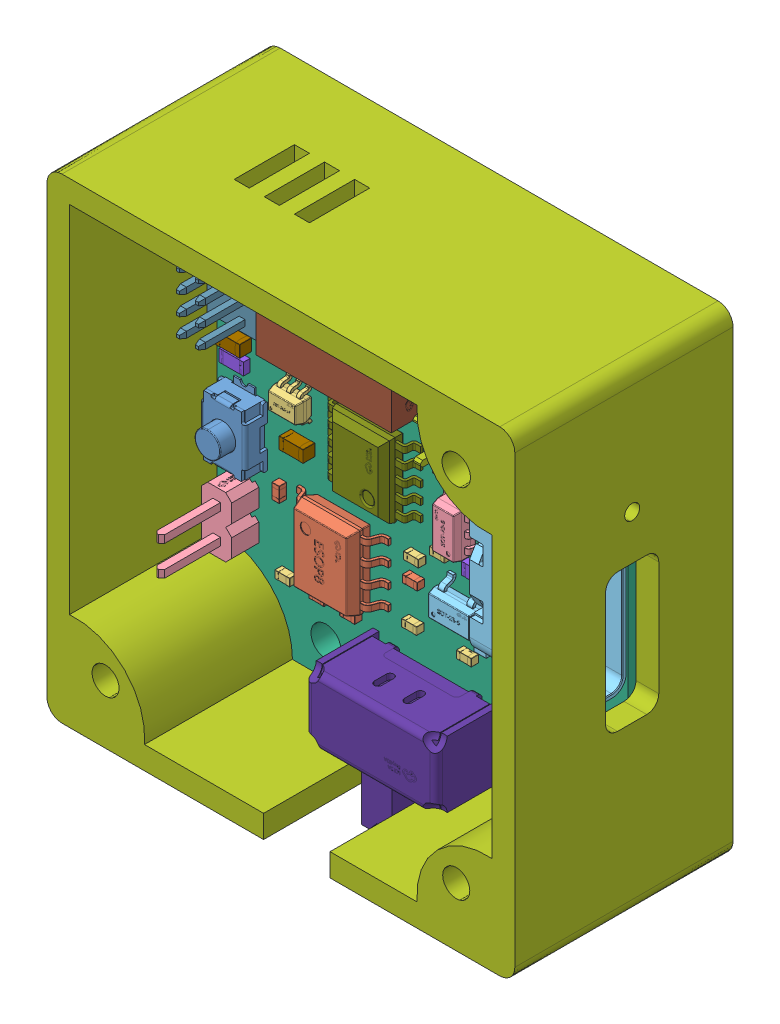
SolidWorks assembly 3D_PCB4_2025-05-12, configuration 默认. Lengths in mm.
Overall size (31.09 33.6 14.5).
127 component instances, 26 part files, 3 mates.
Components (placement in the parent):
- 3D_PCB4_2025-05-12.step-1: 3D_PCB4_2025-05-12.step [默认] at origin size (27.28 31.7 8.7)
  - D4.step-1: D4.step [默认] at (16.256 -9.9568 1.5862) x (-1 0 0) z (0 0 1) size (3.7 1.8 1.14)
    - SOD-123FL_L2.8-W1.8-LS3.7-BI.step-1: SOD-123FL_L2.8-W1.8-LS3.7-BI.step [默认] at origin size (3.7 1.8 1.14)
      - SOLID.step-1: SOLID.step [默认] at origin size (3.7 1.8 1.14)
  - R1.step-1: R1.step [默认] at (4.3814 -18.288 1.5862) x (0 1 0) z (0 0 1) size (1 0.5 0.5)
    - R0402.step-1: R0402.step [默认] at origin size (1 0.5 0.5)
      - SOLID-0.step-1: SOLID-0.step [默认] at origin size (1 0.5 0.5)
  - R2.step-1: R2.step [默认] at (13.305 -18.9963 1.5862) x (-1 0 0) z (0 0 1) size (1 0.5 0.5)
    - R0402.step-1: R0402.step [默认] at origin size (1 0.5 0.5)
      - SOLID-0.step-1: SOLID-0.step [默认] at origin size (1 0.5 0.5)
  - R3.step-1: R3.step [默认] at (20.701 -24.257 1.5862) x (0 -1 0) z (0 0 1) size (1 0.5 0.5)
    - R0402.step-1: R0402.step [默认] at origin size (1 0.5 0.5)
      - SOLID-0.step-1: SOLID-0.step [默认] at origin size (1 0.5 0.5)
  - R4.step-1: R4.step [默认] at (20.701 -26.4161 1.5862) x (0 -1 0) z (0 0 1) size (1 0.5 0.5)
    - R0402.step-1: R0402.step [默认] at origin size (1 0.5 0.5)
      - SOLID-0.step-1: SOLID-0.step [默认] at origin size (1 0.5 0.5)
  - R5.step-1: R5.step [默认] at (7.1031 -22.987 1.5862) size (1 0.5 0.5)
    - R0402.step-1: R0402.step [默认] at origin size (1 0.5 0.5)
      - SOLID-0.step-1: SOLID-0.step [默认] at origin size (1 0.5 0.5)
  - R6.step-1: R6.step [默认] at (9.144 -22.987 1.5862) size (1 0.5 0.5)
    - R0402.step-1: R0402.step [默认] at origin size (1 0.5 0.5)
      - SOLID-0.step-1: SOLID-0.step [默认] at origin size (1 0.5 0.5)
  - R7.step-1: R7.step [默认] at (15.5701 -5.9643 1.5862) x (-1 0 0) z (0 0 1) size (1 0.5 0.5)
    - R0402.step-1: R0402.step [默认] at origin size (1 0.5 0.5)
      - SOLID-0.step-1: SOLID-0.step [默认] at origin size (1 0.5 0.5)
  - R8.step-1: R8.step [默认] at (15.5701 -7.3615 1.5862) x (-1 0 0) z (0 0 1) size (1 0.5 0.5)
    - R0402.step-1: R0402.step [默认] at origin size (1 0.5 0.5)
      - SOLID-0.step-1: SOLID-0.step [默认] at origin size (1 0.5 0.5)
  - C1.step-1: C1.step [默认] at (13.3845 -17.6277 1.5862) x (-1 0 0) z (0 0 1) size (1 0.5 0.5)
    - C0402.step-1: C0402.step [默认] at origin size (1 0.5 0.5)
      - SOLID-1.step-1: SOLID-1.step [默认] at origin size (1 0.5 0.5)
  - C2.step-1: C2.step [默认] at (13.2575 -21.5647 1.5862) x (-1 0 0) z (0 0 1) size (1 0.5 0.5)
    - C0402.step-1: C0402.step [默认] at origin size (1 0.5 0.5)
      - SOLID-1.step-1: SOLID-1.step [默认] at origin size (1 0.5 0.5)
  - C3.step-1: C3.step [默认] at (21.847 -24.257 1.5862) x (0 1 0) z (0 0 1) size (1 0.5 0.5)
    - C0402.step-1: C0402.step [默认] at origin size (1 0.5 0.5)
      - SOLID-1.step-1: SOLID-1.step [默认] at origin size (1 0.5 0.5)
  - C20.step-1: C20.step [默认] at (16.891 -21.5647 1.5862) size (1 0.5 0.5)
    - C0402.step-1: C0402.step [默认] at origin size (1 0.5 0.5)
      - SOLID-1.step-1: SOLID-1.step [默认] at origin size (1 0.5 0.5)
  - C6.step-1: C6.step [默认] at (26.0351 -20.8598 1.5862) x (0 1 0) z (0 0 1) size (1 0.5 0.5)
    - C0402.step-1: C0402.step [默认] at origin size (1 0.5 0.5)
      - SOLID-1.step-1: SOLID-1.step [默认] at origin size (1 0.5 0.5)
  - C7.step-1: C7.step [默认] at (4.826 -22.987 1.5862) x (-1 0 0) z (0 0 1) size (1 0.5 0.5)
    - C0402.step-1: C0402.step [默认] at origin size (1 0.5 0.5)
      - SOLID-1.step-1: SOLID-1.step [默认] at origin size (1 0.5 0.5)
  - C21.step-1: C21.step [默认] at (15.113 -16.4846 1.5862) size (1 0.5 0.5)
    - C0402.step-1: C0402.step [默认] at origin size (1 0.5 0.5)
      - SOLID-1.step-1: SOLID-1.step [默认] at origin size (1 0.5 0.5)
  - H3.step-1: H3.step [默认] at (1.778 -20.6168 1.5862) x (0 1 0) z (0 0 1) size (4.01 2 8.7)
    - HDR-TH_2P-P2.00-V-M.step-1: HDR-TH_2P-P2.00-V-M.step [默认] at origin size (4.01 2 8.7)
      - SOLID-2.step-1: SOLID-2.step [默认] at origin size (4.01 2 8.7)
  - U11.step-1: U11.step [默认] at (16.637 -18.921 1.5862) size (2.9 3.01 1.25)
    - SOT-23-5_L3.0-W1.7-P0.95-LS2.8-BL.step-1: SOT-23-5_L3.0-W1.7-P0.95-LS2.8-BL.step [默认] at origin size (2.9 3.01 1.25)
      - COMPOUND.step-1: COMPOUND.step [默认] at origin size (2.9 3.01 1.25)
  - U9.step-1: U9.step [默认] at (24.892 -7.874 1.5862) x (-1 0 0) z (0 0 1) size (2.1 1.4 0.8)
    - F0805.step-1: F0805.step [默认] at origin size (2.1 1.4 0.8)
      - SOLID-3.step-1: SOLID-3.step [默认] at origin size (2.1 1.4 0.8)
  - H2.step-1: H2.step [默认] at (19.8587 -5.334 1.5862) size (5.09 2 7.2)
    - HDR-TH_4P-P1.27-V-M.step-1: HDR-TH_4P-P1.27-V-M.step [默认] at origin size (5.09 2 7.2)
      - SOLID-4.step-1: SOLID-4.step [默认] at origin size (5.09 2 7.2)
  - H4.step-1: H4.step [默认] at (19.8864 -7.6708 1.5862) size (5.09 2 7.2)
    - HDR-TH_4P-P1.27-V-M.step-1: HDR-TH_4P-P1.27-V-M.step [默认] at origin size (5.09 2 7.2)
      - SOLID-4.step-1: SOLID-4.step [默认] at origin size (5.09 2 7.2)
  - R12.step-1: R12.step [默认] at (17.4966 -16.4846 1.5862) x (-1 0 0) z (0 0 1) size (1.62 0.81 0.45)
    - R0402-1.step-1: R0402-1.step [默认] at origin size (1.62 0.81 0.45)
      - COMPOUND-5.step-1: COMPOUND-5.step [默认] at origin size (1.62 0.81 0.45)
  - R13.step-1: R13.step [默认] at (16.7346 -11.7094 1.5862) x (-1 0 0) z (0 0 1) size (1.62 0.81 0.45)
    - R0402-1.step-1: R0402-1.step [默认] at origin size (1.62 0.81 0.45)
      - COMPOUND-5.step-1: COMPOUND-5.step [默认] at origin size (1.62 0.81 0.45)
  - R14.step-1: R14.step [默认] at (1.397 -12.2844 1.5862) size (1.62 0.81 0.45)
    - R0402-1.step-1: R0402-1.step [默认] at origin size (1.62 0.81 0.45)
      - COMPOUND-5.step-1: COMPOUND-5.step [默认] at origin size (1.62 0.81 0.45)
  - C12.step-1: C12.step [默认] at (1.5009 -11.049 1.5862) x (-1 0 0) z (0 0 1) size (1.6 0.8 0.8)
    - C0402-1.step-1: C0402-1.step [默认] at origin size (1.6 0.8 0.8)
      - SOLID-6.step-1: SOLID-6.step [默认] at origin size (1.6 0.8 0.8)
  - C22.step-1: C22.step [默认] at (5.715 -14.986 1.5862) x (-1 0 0) z (0 0 1) size (1.6 0.8 0.8)
    - C0402-1.step-1: C0402-1.step [默认] at origin size (1.6 0.8 0.8)
      - SOLID-6.step-1: SOLID-6.step [默认] at origin size (1.6 0.8 0.8)
  - D3.step-1: D3.step [默认] at (15.4432 -1.0668 1.5862) size (2.5 1.25 0.95)
    - SOD-323_L1.7-W1.3-LS2.5-FD.step-1: SOD-323_L1.7-W1.3-LS2.5-FD.step [默认] at origin size (2.5 1.25 0.95)
      - COMPOUND-7.step-1: COMPOUND-7.step [默认] at origin size (2.5 1.25 0.95)
  - BUZZER.step-1: BUZZER.step [默认] at (8.89 -5.179 1.5862) x (0 -1 0) z (0 0 1) size (9 9.01 1.81)
    - BUZ-SMD_L9.0-W9.0-P8.00-LS9.3.step-1: BUZ-SMD_L9.0-W9.0-P8.00-LS9.3.step [默认] at origin size (9 9.01 1.81)
      - SOLID-8.step-1: SOLID-8.step [默认] at origin size (9 9.01 1.81)
  - D1.step-1: D1.step [默认] at (24.3141 -21.0153 1.5862) x (0 -1 0) z (0 0 1) size (2.65 1.3 0.95)
    - SOD-323_L1.8-W1.3-LS2.5-RD.step-1: SOD-323_L1.8-W1.3-LS2.5-RD.step [默认] at origin size (2.65 1.3 0.95)
      - SOLID-9.step-1: SOLID-9.step [默认] at origin size (2.65 1.3 0.95)
  - D2.step-1: D2.step [默认] at (22.5852 -21.0153 1.5862) x (0 -1 0) z (0 0 1) size (2.65 1.3 0.95)
    - SOD-323_L1.8-W1.3-LS2.5-RD.step-1: SOD-323_L1.8-W1.3-LS2.5-RD.step [默认] at origin size (2.65 1.3 0.95)
      - SOLID-9.step-1: SOLID-9.step [默认] at origin size (2.65 1.3 0.95)
  - LED1.step-1: LED1.step [默认] at (24.8995 -5.8674 1.5862) size (1 0.51 0.41)
    - LED_0402.step-1: LED_0402.step [默认] at origin size (1 0.51 0.41)
      - COMPOUND-10.step-1: COMPOUND-10.step [默认] at origin size (1 0.51 0.41)
  - U6.step-1: U6.step [默认] at (2.032 -5.842 1.5862) x (0 -1 0) z (0 0 1) size (7.62 3.4 6.3)
    - HDR-TH_12P-P1.27-V-M-R2-C6-S1.27-1.step-1: HDR-TH_12P-P1.27-V-M-R2-C6-S1.27-1.step [默认] at origin size (7.62 3.4 6.3)
      - SOLID-11.step-1: SOLID-11.step [默认] at origin size (7.62 3.4 6.3)
  - Q2.step-1: Q2.step [默认] at (15.4432 -3.6068 1.5862) size (2.8 2.9 1.4)
    - SOT-23-3_L3.0-W1.7-P0.95-LS2.9-BR.step-1: SOT-23-3_L3.0-W1.7-P0.95-LS2.9-BR.step [默认] at origin size (2.8 2.9 1.4)
      - SOLID-12.step-1: SOLID-12.step [默认] at origin size (2.8 2.9 1.4)
  - U12.step-1: U12.step [默认] at (10.6231 -13.3245 1.5862) x (0 1 0) z (0 0 1) size (4.9 6.15 1.45)
    - ESOP-10_L4.9-W3.9-P1.00-LS6.2-BL-EP.step-1: ESOP-10_L4.9-W3.9-P1.00-LS6.2-BL-EP.step [默认] at origin size (4.9 6.15 1.45)
      - COMPOUND-13.step-1: COMPOUND-13.step [默认] at origin size (4.9 6.15 1.45)
  - SW1.step-1: SW1.step [默认] at (14.732 -25.5271 1.5862) size (8.73 8.4 7.51)
    - SW-TH_SK12D07VG3.step-1: SW-TH_SK12D07VG3.step [默认] at origin size (8.73 8.4 7.51)
      - COMPOUND-14.step-1: COMPOUND-14.step [默认] at origin size (8.73 8.4 7.51)
  - Q1.step-1: Q1.step [默认] at (19.939 -21.082 1.5862) size (2.51 2.9 1.05)
    - SOT-23_L2.9-W1.3-P1.90-LS2.4-BR.step-1: SOT-23_L2.9-W1.3-P1.90-LS2.4-BR.step [默认] at origin size (2.51 2.9 1.05)
      - COMPOUND-15.step-1: COMPOUND-15.step [默认] at origin size (2.51 2.9 1.05)
  - U4.step-1: U4.step [默认] at (1.883 -15.748 1.5862) x (0 -1 0) z (0 0 1) size (4.8 3.01 2.52)
    - SW-SMD_L4.0-W3.0-LS4.8.step-1: SW-SMD_L4.0-W3.0-LS4.8.step [默认] at origin size (4.8 3.01 2.52)
      - COMPOUND-16.step-1: COMPOUND-16.step [默认] at origin size (4.8 3.01 2.52)
  - U1.step-1: U1.step [默认] at (8.5362 -19.6013 1.5862) x (0 -1 0) z (0 0 1) size (4.9 6.1 1.7)
    - ESOP-8_L4.9-W3.9-P1.27-LS6.0-BL-EP.step-1: ESOP-8_L4.9-W3.9-P1.27-LS6.0-BL-EP.step [默认] at origin size (4.9 6.1 1.7)
      - COMPOUND-17.step-1: COMPOUND-17.step [默认] at origin size (4.9 6.1 1.7)
  - Q3.step-1: Q3.step [默认] at (5.5407 -12.446 1.5862) size (2 2.11 1.25)
    - SOT-363_L2.0-W1.3-P0.65-LS2.1-BL.step-1: SOT-363_L2.0-W1.3-P0.65-LS2.1-BL.step [默认] at origin size (2 2.11 1.25)
      - COMPOUND-18.step-1: COMPOUND-18.step [默认] at origin size (2 2.11 1.25)
  - D5.step-1: D5.step [默认] at (16.637 -13.9192 1.5862) x (0 1 0) z (0 0 1) size (2.88 2.79 1.64)
    - SOT-23-6_L2.9-W1.6-P0.95-LS2.8-BL.step-1: SOT-23-6_L2.9-W1.6-P0.95-LS2.8-BL.step [默认] at origin size (2.88 2.79 1.64)
      - COMPOUND-19.step-1: COMPOUND-19.step [默认] at origin size (2.88 2.79 1.64)
  - USB1.step-1: USB1.step [默认] at (22.1955 -13.9612 1.5862) x (0 1 0) z (0 0 1) size (8.94 7.75 4.2)
    - USB-C-SMD_TYPEC-304-BCP16.step-1: USB-C-SMD_TYPEC-304-BCP16.step [默认] at origin size (8.94 7.75 4.2)
      - COMPOUND-20.step-1: COMPOUND-20.step [默认] at origin size (8.94 7.75 4.2)
  - COMPOUND-21.step-1: COMPOUND-21.step [默认] at origin size (27.28 27.79 1.59)
- 底壳-1: 底壳 [默认] at (0 0 -2) x (-1 0 0) z (0 0 -1) size (31.09 31.6 14.5)
- 上壳-1: 上壳 [默认] at origin size (31.09 31.6 9.9) (hidden)
Mates (geometry in assembly coordinates):
- 同心5: concentric: cylinder of 3D_PCB4_2025-05-12.step-1/COMPOUND-21.step-1 through (7.24 -25.6501 0) axis (0 0 1) radius 1; cylinder of 底壳-1 through (7.24 -25.6501 5.374) axis (0 0 -1) radius 0.85
- 同心6: concentric: cylinder of 3D_PCB4_2025-05-12.step-1/COMPOUND-21.step-1 through (20.2 -2.16 0) axis (0 0 1) radius 1; cylinder of 底壳-1 through (20.2 -2.16 5.374) axis (0 0 -1) radius 0.85
- 重合2: coincident: plane of 3D_PCB4_2025-05-12.step-1/COMPOUND-21.step-1 through (13.2447 -13.4932 0) normal (0 0 -1); plane of 底壳-1 through (13.2447 -13.4932 0) normal (0 0 1)
